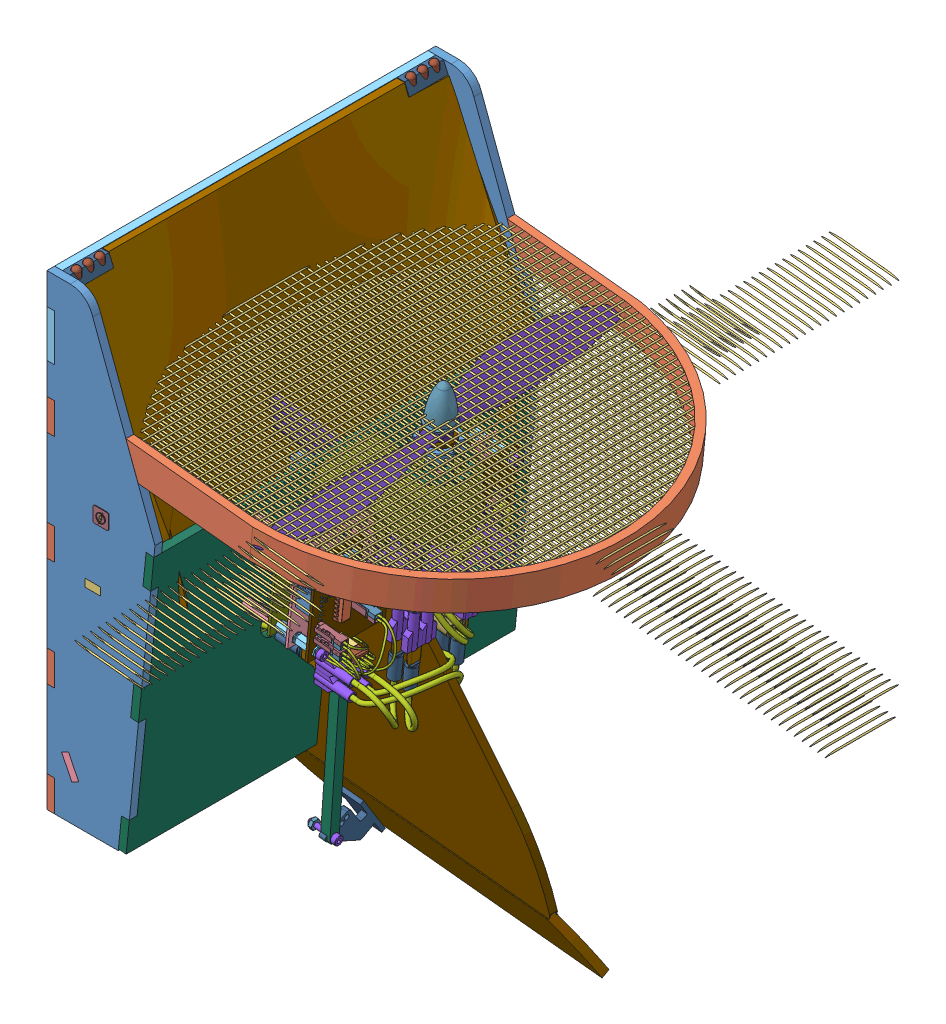
SolidWorks assembly AssTotaleSimu, configuration Défaut. Lengths in mm. (continued)
Components (placement in the parent): (continued)
- AssStructSimu-1: AssStructSimu [Défaut] at (-125.7658 -1.8483 624.6548) x (1 0 0) z (0 0 -1) size (323.53 326.04 251.6) (continued)
  - AssCarte-1: AssCarte [Défaut] at (-42.8534 32.2132 302.028) x (-0.101852 0.9948 0) z (0.9948 0.101852 0) size (91.19 130.57 98.45) (continued)
    - AssCosse-3: AssCosse [Défaut] at (-36.6204 -13.7633 163.5671) x (0 1 0) z (-0.344896 0 0.938641) size (9.83 18.66 11.64) (continued)
      - plain washer 6903 type ab_din-1: plain washer 6903 type ab_din [DIN 6903-A3] at (-2.1064 0.3659 0) size (1 8 8)
      - hex nut style 1 gradeab_din-2: hex nut style 1 gradeab_din [Hexagon Nut ISO 4032 - M3 - W - N] at (1.281 0.3659 0) x (0 0.924225 0.381849) z (-1 0 0) size (5.5 6.35 2.4)
      - 31880-1: 31880 [Default] at (0.4936 0.3659 0) x (0 0.344896 -0.938641) z (0 -0.938641 -0.344896) size (5.54 5 17.37)
    - Terminal_QD_Female-1: Terminal_QD_Female [Default] at (-33.4139 20.2862 128.1409) x (0 1 0) z (-1 0 0) size (9.4 5.5 22.35)
    - Terminal_QD_Female-2: Terminal_QD_Female [Default] at (-33.4139 5.2862 128.1409) x (0 1 0) z (-1 0 0) size (9.4 5.5 22.35)
    - Terminal_QD_Female-3: Terminal_QD_Female [Default] at (-33.4139 -9.7138 128.1409) x (0 1 0) z (-1 0 0) size (9.4 5.5 22.35)
    - Terminal_QD_Female-4: Terminal_QD_Female [Default] at (-33.4139 -9.7138 145.1409) x (0 1 0) z (-1 0 0) size (9.4 5.5 22.35)
    - Terminal_QD_Female-5: Terminal_QD_Female [Default] at (-33.4139 5.2862 145.1409) x (0 1 0) z (-1 0 0) size (9.4 5.5 22.35)
    - Terminal_QD_Female-6: Terminal_QD_Female [Default] at (-33.4139 20.2862 145.1409) x (0 1 0) z (-1 0 0) size (9.4 5.5 22.35)
    - AssCable-2: AssCable [Défaut] at (27.9603 15.7472 146.2789) x (0 1 0) z (-1 0 0) size (18.4 8.94 49.81)
      - 61765-2-1: 61765-2 [Default] at (-1.7839 -0.265 29.3371) size (16.51 3.25 19.56)
      - Terminal_QD_Female-1: Terminal_QD_Female [Default] at (2.5861 -1.0206 32.9742) x (1 0 0) z (0 0 -1) size (9.4 5.5 22.35)
      - Terminal_QD_Female-2: Terminal_QD_Female [Default] at (-6.4139 -1.0206 32.9742) x (1 0 0) z (0 0 -1) size (9.4 5.5 22.35)
      - 141085-2-1: 141085-2 [Default] at (-1.9744 0.1922 19.1771) size (6.91 6.91 25.26)
    - AssCable-3: AssCable [Défaut] at (27.9603 15.7472 136.2789) x (0 1 0) z (-1 0 0) size (18.4 8.94 49.81)
      - 61765-2-1: 61765-2 [Default] at (-1.7839 -0.265 29.3371) size (16.51 3.25 19.56)
      - Terminal_QD_Female-1: Terminal_QD_Female [Default] at (2.5861 -1.0206 32.9742) x (1 0 0) z (0 0 -1) size (9.4 5.5 22.35)
      - Terminal_QD_Female-2: Terminal_QD_Female [Default] at (-6.4139 -1.0206 32.9742) x (1 0 0) z (0 0 -1) size (9.4 5.5 22.35)
      - 141085-2-1: 141085-2 [Default] at (-1.9744 0.1922 19.1771) size (6.91 6.91 25.26)
    - AssCable-4: AssCable [Défaut] at (27.9603 -14.2528 146.2789) x (0 1 0) z (-1 0 0) size (18.4 8.94 49.81)
      - 61765-2-1: 61765-2 [Default] at (-1.7839 -0.265 29.3371) size (16.51 3.25 19.56)
      - Terminal_QD_Female-1: Terminal_QD_Female [Default] at (2.5861 -1.0206 32.9742) x (1 0 0) z (0 0 -1) size (9.4 5.5 22.35)
      - Terminal_QD_Female-2: Terminal_QD_Female [Default] at (-6.4139 -1.0206 32.9742) x (1 0 0) z (0 0 -1) size (9.4 5.5 22.35)
      - 141085-2-1: 141085-2 [Default] at (-1.9744 0.1922 19.1771) size (6.91 6.91 25.26)
    - AssCable-5: AssCable [Défaut] at (27.9603 -14.2528 136.2789) x (0 1 0) z (-1 0 0) size (18.4 8.94 49.81)
      - 61765-2-1: 61765-2 [Default] at (-1.7839 -0.265 29.3371) size (16.51 3.25 19.56)
      - Terminal_QD_Female-1: Terminal_QD_Female [Default] at (2.5861 -1.0206 32.9742) x (1 0 0) z (0 0 -1) size (9.4 5.5 22.35)
      - Terminal_QD_Female-2: Terminal_QD_Female [Default] at (-6.4139 -1.0206 32.9742) x (1 0 0) z (0 0 -1) size (9.4 5.5 22.35)
      - 141085-2-1: 141085-2 [Default] at (-1.9744 0.1922 19.1771) size (6.91 6.91 25.26)
    - AssCable-6: AssCable [Défaut] at (27.005 -44.4196 92.8197) x (0.999998 0.002 0) z (0 0 1) size (18.4 8.94 49.81)
      - 61765-2-1: 61765-2 [Default] at (-1.7839 -0.265 29.3371) size (16.51 3.25 19.56)
      - Terminal_QD_Female-1: Terminal_QD_Female [Default] at (2.5861 -1.0206 32.9742) x (1 0 0) z (0 0 -1) size (9.4 5.5 22.35)
      - Terminal_QD_Female-2: Terminal_QD_Female [Default] at (-6.4139 -1.0206 32.9742) x (1 0 0) z (0 0 -1) size (9.4 5.5 22.35)
      - 141085-2-1: 141085-2 [Default] at (-1.9744 0.1922 19.1771) size (6.91 6.91 25.26)
    - AssCable-7: AssCable [Défaut] at (27.005 -34.4196 92.8197) x (0.999998 0.002 0) z (0 0 1) size (18.4 8.94 49.81)
      - 61765-2-1: 61765-2 [Default] at (-1.7839 -0.265 29.3371) size (16.51 3.25 19.56)
      - Terminal_QD_Female-1: Terminal_QD_Female [Default] at (2.5861 -1.0206 32.9742) x (1 0 0) z (0 0 -1) size (9.4 5.5 22.35)
      - Terminal_QD_Female-2: Terminal_QD_Female [Default] at (-6.4139 -1.0206 32.9742) x (1 0 0) z (0 0 -1) size (9.4 5.5 22.35)
      - 141085-2-1: 141085-2 [Default] at (-1.9744 0.1922 19.1771) size (6.91 6.91 25.26)
    - 281838-3-1: 281838-3 [Default] at (-0.2889 -49.1668 143.7439) x (0 -1 0) z (0 0 1) size (7.62 5.3 15)
    - 165085-1: 165085 [Default] at (-0.9405 -5.6672 127.3501) x (-0.869274 0.49433 0) z (0 0 -1) size (7.09 7.09 28.56)
    - 165085-2: 165085 [Default] at (-0.9405 -0.6672 127.3501) x (-0.869274 0.49433 0) z (0 0 -1) size (7.09 7.09 28.56)
    - 661002113322_Downloads_STP_661002113322_rev1-1: 661002113322_Downloads_STP_661002113322_rev1 [Défaut] at (-11.9389 -60.1918 128.7439) x (1 0 0) z (0 -1 0) size (5.08 14.61 5.18)
      - 48532480_02_03_04_05_08_10_740_DX-1: 48532480_02_03_04_05_08_10_740_DX [Défaut] at (-2.54 0 0) size (2.54 14.61 5.18)
      - 48532480_02_03_04_05_08_10_740_SX-1: 48532480_02_03_04_05_08_10_740_SX [Défaut] at origin size (2.54 14.61 5.18)
    - 661002113322_Downloads_STP_661002113322_rev1-2: 661002113322_Downloads_STP_661002113322_rev1 [Défaut] at (-21.5488 -42.0726 128.7439) x (-1 0 0) z (0 1 0) size (5.08 14.61 5.18)
      - 48532480_02_03_04_05_08_10_740_DX-1: 48532480_02_03_04_05_08_10_740_DX [Défaut] at (-2.54 0 0) size (2.54 14.61 5.18)
      - 48532480_02_03_04_05_08_10_740_SX-1: 48532480_02_03_04_05_08_10_740_SX [Défaut] at origin size (2.54 14.61 5.18)
    - 661002113322_Downloads_STP_661002113322_rev1-3: 661002113322_Downloads_STP_661002113322_rev1 [Défaut] at (-5.6389 -60.1918 128.7439) x (1 0 0) z (0 -1 0) size (5.08 14.61 5.18)
      - 48532480_02_03_04_05_08_10_740_DX-1: 48532480_02_03_04_05_08_10_740_DX [Défaut] at (-2.54 0 0) size (2.54 14.61 5.18)
      - 48532480_02_03_04_05_08_10_740_SX-1: 48532480_02_03_04_05_08_10_740_SX [Défaut] at origin size (2.54 14.61 5.18)
- AssTige-1: AssTige [Défaut] at (-241.576 -121.7726 340.4233) x (-0.101791 -0.994204 -0.034587) z (0.9948 -0.101852 0) size (166.39 7.19 19)
  - tige_servo-1: tige_servo [Défaut] at (-106.2712 0.2685 162) size (165 6 6)
  - socket head cap screw 4762_din-2: socket head cap screw 4762_din [EN ISO 4762 M2 x 10 - 10N] at (-104.2712 3.2685 170) x (0 0 -1) z (0.923728 0.383049 0) size (12 3.8 3.8)
  - hex nut style 1 gradeab_din-1: hex nut style 1 gradeab_din [Hexagon Nut ISO 4032 - M3 - W - N] at (55.7288 3.2685 156) size (5.5 6.35 2.4)
  - hex nut style 1 gradeab_din-2: hex nut style 1 gradeab_din [Hexagon Nut ISO 4032 - M2 - W - N] at (-104.2712 3.2685 160) x (0.904801 0.425836 0) z (0 0 1) size (4 4.62 1.6)
  - socket head cap screw 4762_din-3: socket head cap screw 4762_din [EN ISO 4762 M3 x 16 - 16N] at (55.7288 3.2685 171) x (0 0 -1) z (0.923728 0.383049 0) size (19 5.5 5.5)
- AssGoPro-1: AssGoPro [Défaut] at (-119.9926 15.1708 318.2917) x (0 0 -1) z (-0.119031 -0.99289 0) size (64.3 52.3 34.42)
  - GoPRo Frame for LCD Screen-1: GoPRo Frame for LCD Screen [Défaut] at (-2.6935 10.9558 5.5635) size (64.3 59.3 34.42)
    - GoProFrame MJM-1: GoProFrame MJM [Défaut] at (-3.6084 -1.6692 52.45) size (64.3 47.42 23.68)
    - GoPro Hero 3 Front Panel-1: GoPro Hero 3 Front Panel [Défaut] at (-3.6084 -1.6692 55.7) x (-1 0 0) z (0 0 -1) size (59.25 41.2 1.9)
    - GoPro Hero 3 Screen-1: GoPro Hero 3 Screen [Défaut] at (12.7166 3.9308 54.9) size (15 18 1)
    - GoPro Hero 3 Mode Button-1: GoPro Hero 3 Mode Button [Défaut] at (13.4166 -12.4692 54.95) x (-1 0 0) z (0 0 -1) size (11.97 12.11 3.03)
    - GoPro Hero 3 LED Cover-1: GoPro Hero 3 LED Cover [Défaut] at (3.1166 -9.3192 54.85) x (-0.999988 0.004848 0) z (0 0 -1) size (5 5 1.4)
    - GoPro Hero 3 LED Cover-2: GoPro Hero 3 LED Cover [Défaut] at (3.1166 -16.0692 54.85) x (-0.999988 0.004848 0) z (0 0 -1) size (5 5 1.4)
    - GoPro Hero 3 Housing-1: GoPro Hero 3 Housing [Défaut] at (-3.6084 -1.6692 55.7) size (59.37 41.3 29.84)
    - GoPro Hero 3 Lens-1: GoPro Hero 3 Lens [Défaut] at (-18.9334 5.6308 47.35) x (-0.380542 -0.924764 0) z (0 0 -1) size (13.71 15.7 7.94)
    - GoPro Hero 3 Indicator Cover-1: GoPro Hero 3 Indicator Cover [Défaut] at (-25.5834 -22.2692 69.9) x (-0.997412 0 -0.0719) z (0 1 0) size (3 3 2)
    - GoPro Hero 3 Indicator Cover-2: GoPro Hero 3 Indicator Cover [Défaut] at (-28.8834 12.2308 73) x (-0.999992 0.004018 0) z (0 0 1) size (3 3 2)
    - GoPro Hero 3 Indicator Cover-3: GoPro Hero 3 Indicator Cover [Défaut] at (20.6666 16.9308 58.4) x (-0.997739 0 -0.067212) z (0 1 0) size (3 3 2)
    - slot-1: slot [Défaut] at (-24.7434 -9.7363 65.05) x (0 1 0) z (0 0 -1) size (16 15.02 2.44)
    - GoPro Hero 3 HDMI pin-1: GoPro Hero 3 HDMI pin [Défaut] at (-26.982 2.9815 24.7172) x (0.105491 0.98175 -0.158237) z (-0.992872 0.095109 -0.071829) size (3.29 0.86 3.28)
  - support1-2: support1 [Défaut] at (-1.3019 -18.8633 67.0135) x (0 0 1) z (-1 0 0) size (5 5 10)
- AssGouv-1: AssGouv [Défaut] at (-43.2668 -298.2106 479.8345) x (0.9948 -0.101852 0) z (0.055947 0.546439 -0.835628) size (200.18 52.5 43.47)
  - P10_1-1: P10_1 [Défaut] at (-108.1667 -19.4144 197.6829) size (200.18 50.13 5)
  - attache_pale-1: attache_pale [Défaut] at (-49.1667 8.0856 190.1829) x (0 0 -1) z (-1 0 0) size (43.47 35 14)
- Parallax-Servo-Horn-1: Parallax-Servo-Horn [Défaut] at (-69.3162 -29.8353 324.5606) x (0.09792 0.956393 0.27518) z (0.9948 -0.101852 0) size (38.81 38.81 6.17)
- NTM_35-36_engine_assembly-1: NTM_35-36_engine_assembly [Défaut] at (-28.31 27.2833 324.0336) x (-0.956606 0.097941 0.274431) z (-0.273004 0.027951 -0.961607) size (60.56 77.2 246.41)
  - engine_base-1: engine_base [Défaut] at (-1.8719 -19.5526 -1.1165) x (0 1 0) z (0 0 1) size (6.8 35 35)
  - engine_bearing-1: engine_bearing [Défaut] at origin size (10 4 10)
  - Propeller_cone-1: Propeller_cone [Défaut] at (-1.8719 33.6474 -4.1165) x (1 0 0) z (0 1 0) size (17.6 17.6 24)
  - engine_bearing-2: engine_bearing [Défaut] at (0 22.8 0) size (10 4 10)
  - NTM_35-36_enginebody-1: NTM_35-36_enginebody [Défaut] at (-1.8719 -12.7526 -1.1165) size (35 31.7 35)
  - Stator-1: Stator [Défaut] at origin size (27.75 22.36 27.94)
  - propellers_10x4-1: propellers_10x4 [Défaut] at (-6.8719 27.4474 -4.9165) size (60.56 10.53 246.41)
  - propeller_washer-1: propeller_washer [Défaut] at (-1.8719 24.4474 -1.1165) x (0 1 0) z (0 0 1) size (2.5 18 18)
  - Propeller_adaptor-1: Propeller_adaptor [Défaut] at (2.1948 17.1101 -3.713) size (23.46 32.5 25)
Mates (geometry in assembly coordinates):
- Coaxiale1: concentric aligned: cylinder of AssStructSimu-1/AssToitMot-1/AssToit-1/P12-1 through (-27.6967 12.5918 324.5936) axis (-0.101852 -0.9948 0) radius 17.5; cylinder of NTM_35-36_engine_assembly-1/NTM_35-36_enginebody-1 through (-25.2217 36.7654 324.5936) axis (-0.101852 -0.9948 0) radius 17.5
- Coïncidente1: coincident anti-aligned: plane of AssStructSimu-1/AssToitMot-1/AssToit-1/P12-1 through (-28.206 7.6178 324.5936) normal (0.101852 0.9948 0); plane of NTM_35-36_engine_assembly-1/engine_bearing-1 through (-28.206 7.6178 324.5936) normal (-0.101852 -0.9948 0)
- Coaxiale2: concentric aligned: cylinder of AssStructSimu-1/AssToitMot-1/AssToit-1/P10_2-1 through (49.7135 -178.7878 324.5936) axis (-0.9948 0.101852 0) radius 2.5; cylinder of AssGouv-1/P10_1-1 through (-94.0351 -164.0702 324.5936) axis (-0.9948 0.101852 0) radius 2.5
- Coïncidente2: coincident aligned: plane of AssStructSimu-1/AssToitMot-1/AssToit-1/P10_2-1 through (-137.5516 -157.1017 322.0936) normal (-0.9948 0.101852 0); plane of AssGouv-1/P10_1-1 through (-137.8791 -160.3008 321.1312) normal (-0.9948 0.101852 0)
- Coaxiale3: concentric aligned: cylinder of AssTige-1/socket head cap screw 4762_din-3 through (-45.5416 -197.7164 335.2292) axis (0.9948 -0.101852 0) radius 1.5; cylinder of AssGouv-1/attache_pale-1 through (-85.9983 -193.5742 335.2292) axis (0.9948 -0.101852 0) radius 1.5
- Coaxiale4: concentric aligned: cylinder of AssStructSimu-1/AssToitMot-1/Parallax-Servo_DUMMY-1 through (-70.6554 -29.6982 324.5606) axis (-0.9948 0.101852 0) radius 2.9845; cylinder of Parallax-Servo-Horn-1 through (-70.6554 -29.6982 324.5606) axis (-0.9948 0.101852 0) radius 2.9845
- Coïncidente3: coincident anti-aligned: plane of AssStructSimu-1/AssToitMot-1/Parallax-Servo_DUMMY-1 through (-74.8246 -29.2713 324.5606) normal (0.9948 -0.101852 0); plane of Parallax-Servo-Horn-1 through (-74.8246 -29.2713 324.5606) normal (-0.9948 0.101852 0)
- Coaxiale5: concentric anti-aligned: cylinder of AssTige-1/socket head cap screw 4762_din-2 through (-30.2498 -38.5418 340.7631) axis (0.9948 -0.101852 0) radius 1; cylinder of Parallax-Servo-Horn-1 through (-69.7931 -34.4932 340.7631) axis (-0.9948 0.101852 0) radius 0.635
- Coïncidente4: coincident anti-aligned: plane of AssTige-1/tige_servo-1 through (-69.6001 -32.608 343.8305) normal (-0.9948 0.101852 0); plane of Parallax-Servo-Horn-1 through (-68.8748 -25.5237 332.3708) normal (0.9948 -0.101852 0)
- Coaxiale6: concentric aligned: cylinder of AssStructSimu-1/AssBase-1/socket head cap screw 4762_din-7 through (-144.5139 -51.9008 369.3436) axis (0 0 1) radius 1.5; cylinder of AssGoPro-1/support1-2 through (-144.5139 -51.9008 319.5936) axis (0 0 1) radius 1.5
- Coïncidente5: coincident anti-aligned: plane of AssStructSimu-1/AssBase-1/support2-1 through (-141.9706 -54.3568 329.5936) normal (0 0 -1); plane of AssGoPro-1/support1-2 through (-146.6985 -49.121 329.5936) normal (0 0 1)
